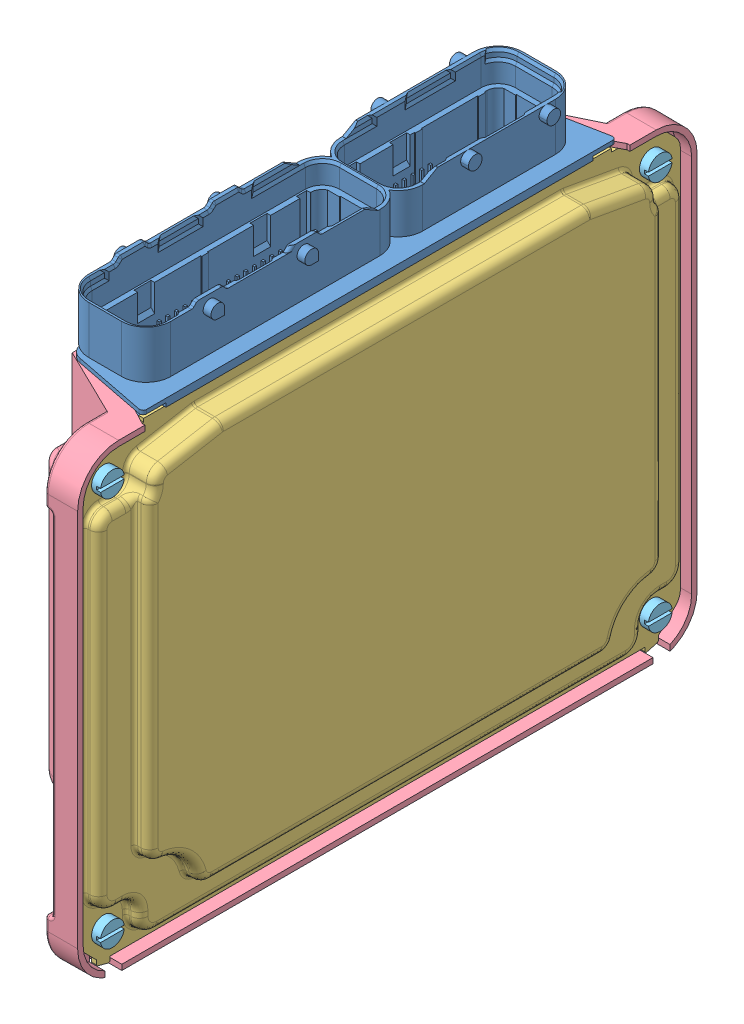
SolidWorks assembly volkwagen b covers, configuration По умолчанию. Lengths in mm.
Overall size (38.95 151.82 181.5).
11 component instances, 5 part files, 0 mates.
Components (placement in the parent):
- volkwagen b covers.stp-1: volkwagen b covers.stp [По умолчанию] at origin size (38.95 151.82 181.5)
  - GDI-4ch 1.stp-1: GDI-4ch 1.stp [По умолчанию] at (4 -58.4831 -82) x (0 0 1) z (-1 0 0) size (164 142.81 36.19)
    - TE_368255-2.stp-1: TE_368255-2.stp [По умолчанию] at (82.042 141.478 18.65) x (-1 0 0) z (0 1 0) size (144 36.19 46.33)
      - SOLID.stp-1: SOLID.stp [По умолчанию] at origin size (144 36.19 46.33)
    - GDI-4ch PCB.stp-1: GDI-4ch PCB.stp [По умолчанию] at origin size (164 118 1.6)
  - eBom-prt2.stp-1: eBom-prt2.stp [По умолчанию] at origin size (10 133 177.5)
  - eBom-prt3.stp-1: eBom-prt3.stp [По умолчанию] at (-24.6 0 0) size (29.01 135 181.5)
  - eBom-prt4.stp-1: eBom-prt4.stp [По умолчанию] at (1.5 -57.1 -80.25) x (-1 0 0) z (0 0 -1) size (8.6 7 7)
  - eBom-prt4.stp-2: eBom-prt4.stp [По умолчанию] at (1.5 57.1 -80.25) x (-1 0 0) z (0 0 -1) size (8.6 7 7)
  - eBom-prt4.stp-3: eBom-prt4.stp [По умолчанию] at (1.5 -57.1 80.25) x (-1 0 0) z (0 0 -1) size (8.6 7 7)
  - eBom-prt4.stp-4: eBom-prt4.stp [По умолчанию] at (1.5 57.1 80.25) x (-1 0 0) z (0 0 -1) size (8.6 7 7)
